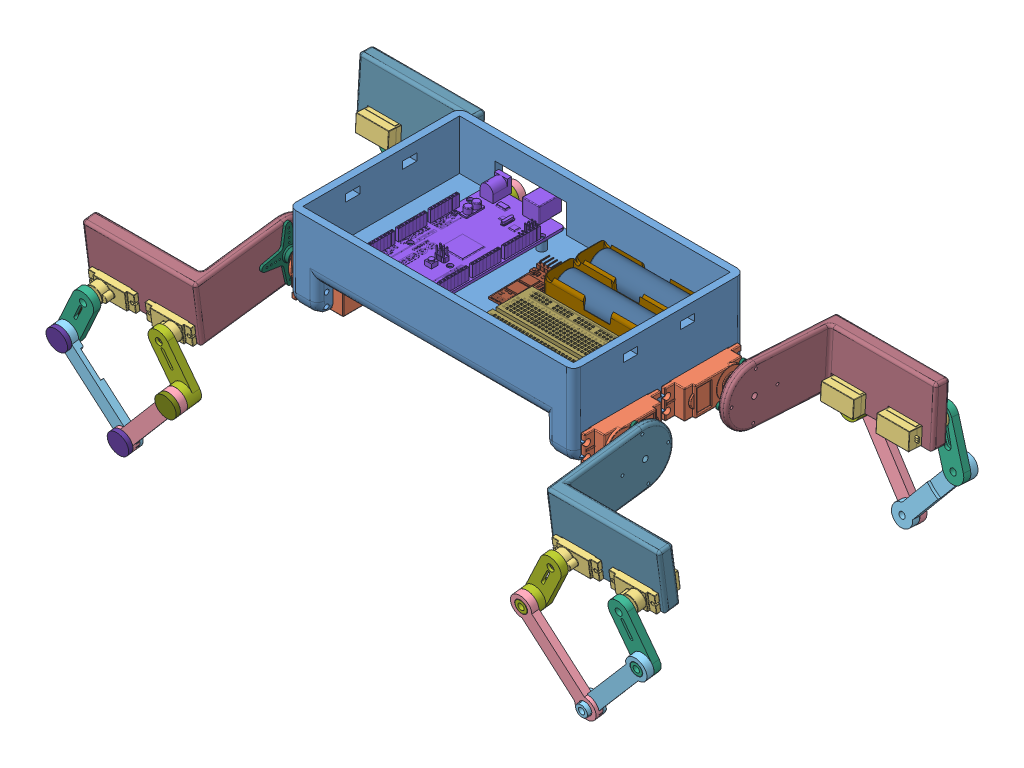
SolidWorks assembly ASSY2, configuration Default. Lengths in mm.
Overall size (425 157.55 250.82).
49 component instances, 18 part files, 74 mates.
Components (placement in the parent):
- part1-1: part1 [Default] at (0 551.341 0) size (200.21 60 120)
- Servo MG996R-2: Servo MG996R [Predeterminado] at (-73.4 551.341 48.3) x (0 0 -1) z (0 1 0) size (53.6 47.6 20)
- Servo-MG90S-1: Servo-MG90S [Default] at (-142.75 521.5824 79.9275) x (1 0 0) z (0 -0.991575 -0.129534) size (32.2 32.5 12.4)
- Servo-MG90S-2: Servo-MG90S [Default] at (-182.75 521.5824 79.9275) x (-1 0 0) z (0 0.991575 0.129534) size (32.2 32.5 12.4)
- legpart1-1: legpart1 [Default] at (-123.3346 490.3083 115.1734) x (-0.653604 -0.75046 -0.098036) z (0 -0.129534 0.991575) size (75 15 5)
- legpart2-1: legpart2 [Default] at (-201.9182 490.4764 112.8758) x (0.656123 -0.748296 -0.097754) z (0 -0.129534 0.991575) size (75 15 10)
- legpart3-1: legpart3 [Default] at (-188 517.4761 111.3604) x (-0.46394 -0.878403 -0.11475) z (0 -0.129534 0.991575) size (45 15 10)
- legpart4-1: legpart4 [Default] at (-137.5 517.8259 108.6831) x (0.472181 -0.874075 -0.114185) z (0 -0.129534 0.991575) size (45 15 15.1)
- Arduino Mega.step-1: Arduino Mega.step [Default] at (-11.5076 562.341 34.714) x (0.34202 0 -0.939693) z (0.939693 0 0.34202) size (114.59 14.37 81.93)
  - ARDUINO MEGA_1.step-1: ARDUINO MEGA_1.step [Default] at origin size (114.59 14.37 81.93)
- 18650BatteryCase v6.step-1: 18650BatteryCase v6.step [Default] at (12.6809 556.341 -27.3839) x (1 0 0) z (0 1 0) size (76.1 23.18 18.4)
- 18650 battery-1: 18650 battery [Default] at (82.6809 566.341 -39.3839) x (0 0 1) z (0 -1 0) size (18.4 65 18.4)
- 18650 battery-3: 18650 battery [Default] at (82.6809 566.341 -15.3839) x (0 0 -1) z (0 1 0) size (18.4 65 18.4)
- 18650BatteryCase v6.step-3: 18650BatteryCase v6.step [Default] at (12.6809 556.341 -5.8839) x (1 0 0) z (0 1 0) size (76.1 23.18 18.4)
- HC-05-1: HC-05 [Default] at (-0.9997 556.341 -7.5776) x (-0.021576 0 -0.999767) z (0.999767 0 -0.021576) size (42.58 6.55 16)
- matrix-1: matrix [Default] at (54 556.341 28.5) size (82 14.01 53)
- part2L-7: part2L [Default] at (-125.75 541.341 38.3) x (0 -0.129534 0.991575) z (-1 0 0) size (82.34 40 80)
- part2R-7: part2R [Default] at (-125.75 541.341 -38.3) x (0 -0.058757 -0.998272) z (-1 0 0) size (82.34 40 80)
- Servo MG996R-8: Servo MG996R [Predeterminado] at (-73.4 531.341 -48.3) x (0 0 1) z (0 -1 0) size (53.6 47.6 20)
- Servo MG996R-9: Servo MG996R [Predeterminado] at (73.4 551.341 -48.3) x (0 0 1) z (0 1 0) size (53.6 47.6 20)
- Servo MG996R-10: Servo MG996R [Predeterminado] at (73.4 531.341 48.3) x (0 0 -1) z (0 -1 0) size (53.6 47.6 20)
- Servo Control Horns-1: Servo Control Horns [4 Arm] at (-121 531.0968 37.9577) x (0 -0.999442 -0.033391) z (-1 0 0) size (39 39 5.5)
- Servo Control Horns-2: Servo Control Horns [4 Arm] at (-121 540.9638 -28.057) x (0 -0.036806 0.999322) z (-1 0 0) size (39 39 5.5)
- Servo-MG90S-13: Servo-MG90S [Default] at (-182.75 524.5899 -81.2261) x (-1 0 0) z (0 -0.998272 0.058757) size (32.2 32.5 12.4)
- Servo-MG90S-14: Servo-MG90S [Default] at (-143.75 524.5899 -81.2261) x (1 0 0) z (0 0.998272 -0.058757) size (32.2 32.5 12.4)
- legpart4-8: legpart4 [Default] at (-138.5 522.8859 -110.176) x (0.476344 -0.87774 0.051662) z (0 -0.058757 -0.998272) size (45 15 15.1)
- legpart1-8: legpart1 [Default] at (-124.2097 495.6724 -123.6002) x (-0.593927 -0.803129 0.047271) z (0 0.058757 0.998272) size (75 15 5)
- legpart2-8: legpart2 [Default] at (-197.9499 494.3391 -113.5044) x (0.635076 -0.771115 0.045387) z (0 -0.058757 -0.998272) size (75 15 10)
- legpart3-8: legpart3 [Default] at (-188 522.8859 -110.176) x (-0.331664 -0.941768 0.055431) z (0 -0.058757 -0.998272) size (45 15 10)
- Servo Control Horns-3: Servo Control Horns [4 Arm] at (121 551.5745 -37.7196) x (0 0.998396 0.056621) z (1 0 0) size (39 39 5.5)
- Servo Control Horns-5: Servo Control Horns [4 Arm] at (121 541.7183 28.057) x (0 0.036806 -0.999322) z (1 0 0) size (39 39 5.5)
- part2R-12: part2R [Default] at (125.75 541.341 38.3) x (0 -0.129534 0.991575) z (1 0 0) size (82.34 40 80)
- part2L-13: part2L [Default] at (125.75 541.341 -38.3) x (0 -0.058757 -0.998272) z (1 0 0) size (82.34 40 80)
- legpart4-14: legpart4 [Default] at (138.5 522.8859 -110.176) x (-0.476344 -0.87774 0.051662) z (0 -0.058757 -0.998272) size (45 15 15.1)
- legpart3-14: legpart3 [Default] at (188 522.8859 -110.176) x (0.331664 -0.941768 0.055431) z (0 -0.058757 -0.998272) size (45 15 10)
- Servo-MG90S-25: Servo-MG90S [Default] at (182.75 524.5899 -81.2261) x (1 0 0) z (0 0.998272 -0.058757) size (32.2 32.5 12.4)
- Servo-MG90S-26: Servo-MG90S [Default] at (143.75 524.5899 -81.2261) x (-1 0 0) z (0 -0.998272 0.058757) size (32.2 32.5 12.4)
- legpart1-14: legpart1 [Default] at (124.2097 495.9662 -118.6089) x (0.593927 -0.803129 0.047271) z (0 -0.058757 -0.998272) size (75 15 5)
- legpart2-14: legpart2 [Default] at (197.9499 494.3391 -113.5044) x (-0.635076 -0.771115 0.045387) z (0 -0.058757 -0.998272) size (75 15 10)
- Servo-MG90S-27: Servo-MG90S [Default] at (142.75 521.5824 79.9275) x (-1 0 0) z (0 0.991575 0.129534) size (32.2 32.5 12.4)
- Servo-MG90S-28: Servo-MG90S [Default] at (182.75 521.5824 79.9275) x (1 0 0) z (0 -0.991575 -0.129534) size (32.2 32.5 12.4)
- legpart3-15: legpart3 [Default] at (188 517.4761 111.3604) x (0.46394 -0.878403 -0.11475) z (0 -0.129534 0.991575) size (45 15 10)
- legpart2-15: legpart2 [Default] at (201.9182 490.4764 112.8758) x (-0.656123 -0.748296 -0.097754) z (0 -0.129534 0.991575) size (75 15 10)
- legpart1-15: legpart1 [Default] at (123.3346 489.6606 120.1312) x (0.653604 -0.75046 -0.098036) z (0 0.129534 -0.991575) size (75 15 5)
- legpart4-15: legpart4 [Default] at (137.5 517.8259 108.6831) x (-0.472181 -0.874075 -0.114185) z (0 -0.129534 0.991575) size (45 15 15.1)
- legpart5-1: legpart5 [Default] at (-123.3346 489.272 123.106) x (-0.914565 -0.401032 -0.052389) z (0.40444 -0.906859 -0.118467) size (15 18 15)
- legpart6-1: legpart6 [Default] at (-162.5508 444.2444 117.2238) x (0.999961 0.008715 0.001138) z (-0.008789 0.991537 0.129529) size (15 13 15)
- legpart6-2: legpart6 [Default] at (-201.9182 489.4401 120.8084) x (0.324849 0.937798 0.122509) z (-0.945766 0.322112 0.042079) size (15 13 15)
- servo horn 1 v2.step-1: servo horn 1 v2.step [Default] at (-188 517.3725 112.1537) x (0.877073 -0.476309 -0.062223) z (-0.480356 -0.869684 -0.113611) size (7.2 3.7 21.2)
Mates (geometry in assembly coordinates):
- 일치5: coincident: plane of part1-1 through (0 551.341 0) normal (0 -1 0); plane of Servo MG996R-2 through (-110 551.341 48.3) normal (0 1 0)
- 일치22: coincident: plane of Servo-MG90S-1 through (-137.5 517.8259 108.6831) normal (0 -0.129534 0.991575); plane of legpart4-1 through (-137.5 517.8259 108.6831) normal (0 0.129534 -0.991575)
- 동심5: concentric: cylinder of Servo-MG90S-1 through (-137.5 517.6963 109.6747) axis (0 -0.129534 0.991575) radius 1.25; cylinder of legpart4-1 through (-137.5 517.1782 113.641) axis (0 0.129534 -0.991575) radius 2.5
- 동심6: concentric: cylinder of legpart1-1 through (-123.3346 489.6606 120.1312) axis (0 0.129534 -0.991575) radius 4.5; cylinder of legpart4-1 through (-123.3346 489.6476 120.2304) axis (0 0.129534 -0.991575) radius 4.25
- 일치23: coincident: plane of legpart1-1 through (-123.3346 490.3083 115.1734) normal (0 0.129534 -0.991575); plane of legpart4-1 through (-123.3346 490.3083 115.1734) normal (0 -0.129534 0.991575)
- 동심7: concentric: cylinder of Servo-MG90S-2 through (-188 517.6963 109.6747) axis (0 -0.129534 0.991575) radius 1.25; cylinder of legpart3-1 through (-188 516.8285 116.3183) axis (0 0.129534 -0.991575) radius 2.5
- 동심8: concentric: cylinder of legpart2-1 through (-201.9182 489.8287 117.8336) axis (0 0.129534 -0.991575) radius 4.5; cylinder of legpart3-1 through (-201.9182 489.8287 117.8336) axis (0 0.129534 -0.991575) radius 4.25
- 일치25: coincident: plane of legpart2-1 through (-201.9182 490.4764 112.8758) normal (0 0.129534 -0.991575); plane of legpart3-1 through (-188 516.8285 116.3183) normal (0 -0.129534 0.991575)
- 동심9: concentric: cylinder of legpart1-1 through (-162.5508 444.633 114.2491) axis (0 0.129534 -0.991575) radius 4.5; cylinder of legpart2-1 through (-162.5508 444.2832 116.9263) axis (0 0.129534 -0.991575) radius 4.25
- 거리7: distance = 20 mm: plane of Arduino Mega.step-1/ARDUINO MEGA_1.step-1 through (-40 564.141 -52) normal (-1 0 0); plane of part1-1 through (-20 576.341 -45) normal (-1 0 0)
- 일치31: coincident: plane of part1-1 through (0 556.341 0) normal (0 1 0); plane of 18650BatteryCase v6.step-1 through (50.6809 556.341 -38.1339) normal (0 -1 0)
- 거리8: distance = 10 mm: plane of 18650BatteryCase v6.step-1 through (12.6809 556.341 -27.3839) normal (0 1 0); plane of 18650 battery-1 through (82.6809 566.341 -39.3839) normal (0 -1 0)
- 거리9: distance = 12 mm: plane of 18650 battery-1 through (82.6809 566.341 -39.3839) normal (0 0 1); plane of 18650BatteryCase v6.step-1 through (12.6809 556.341 -27.3839) normal (0 0 -1)
- 거리10: distance = 70 mm: plane of 18650 battery-1 through (82.6809 566.341 -39.3839) normal (-1 0 0); plane of 18650BatteryCase v6.step-1 through (12.6809 556.341 -27.3839) normal (1 0 0)
- 일치33: coincident: plane of part1-1 through (0 556.341 0) normal (0 1 0); plane of matrix-1 through (54 556.341 28.5) normal (0 -1 0)
- 일치34: coincident: plane of part1-1 through (95 591.341 -55) normal (-1 0 0); plane of matrix-1 through (95 570.3451 2) normal (1 0 0)
- 일치35: coincident: plane of part1-1 through (-95 591.341 55) normal (0 0 -1); plane of matrix-1 through (95 570.3451 55) normal (0 0 1)
- 일치36: coincident: plane of part1-1 through (0 556.341 0) normal (0 1 0); plane of HC-05-1 through (-0.9997 556.341 -7.5776) normal (0 -1 0)
- 일치38: coincident: plane of part1-1 through (0 551.341 0) normal (1 0 0); plane of assembly through (0 0 0) normal (1 0 0)
- 일치39: coincident: plane of part1-1 through (-100 556.341 -60) normal (0 0 -1); plane of Arduino Mega.step-1/ARDUINO MEGA_1.step-1 through (-34 564.641 -60) normal (0 0 -1)
- 일치40: coincident: plane of part1-1 through (-62.5 562.341 12.1502) normal (0 1 0); plane of Arduino Mega.step-1/ARDUINO MEGA_1.step-1 through (-44 562.341 -52) normal (0 -1 0)
- 일치42: coincident: plane of Servo-MG90S-2 through (-182.75 519.186 98.2716) normal (0 0.129534 -0.991575); plane of part2L-7 through (-125.75 533.2663 100.111) normal (0 -0.129534 0.991575)
- 일치44: coincident: plane of Servo-MG90S-2 through (-182.75 527.7301 80.7306) normal (0 0.991575 0.129534); plane of part2L-7 through (-194.75 526.6291 89.159) normal (0 -0.991575 -0.129534)
- 일치45: coincident: plane of Servo-MG90S-1 through (-142.75 527.7301 80.7306) normal (0 0.991575 0.129534); plane of part2L-7 through (-130.75 526.6291 89.159) normal (0 -0.991575 -0.129534)
- 일치46: coincident: plane of Servo-MG90S-1 through (-142.75 519.186 98.2716) normal (0 0.129534 -0.991575); plane of part2L-7 through (-125.75 533.2663 100.111) normal (0 -0.129534 0.991575)
- 거리11: distance = 0.5 mm: plane of Servo-MG90S-1 through (-154.25 513.2365 97.4944) normal (-1 0 0); plane of part2L-7 through (-154.75 514.7302 87.6046) normal (1 0 0)
- 거리12: distance = 0.5 mm: plane of part2L-7 through (-194.75 514.7302 87.6046) normal (1 0 0); plane of Servo-MG90S-2 through (-194.25 525.1354 99.0488) normal (-1 0 0)
- 동심14: concentric: cylinder of Servo MG996R-2 through (-114.1 541.341 38.3) axis (-1 0 0) radius 1.3; cylinder of Servo Control Horns-1 through (-122.75 541.341 38.3) axis (1 0 0) radius 1.25
- 일치47: coincident: plane of Servo MG996R-2 through (-121 541.341 38.3) normal (-1 0 0); plane of Servo Control Horns-1 through (-121 531.0968 37.9577) normal (1 0 0)
- 일치48: coincident: plane of part2L-7 through (-122.75 541.341 38.3) normal (1 0 0); plane of Servo Control Horns-1 through (-122.75 531.0968 37.9577) normal (-1 0 0)
- 동심16: concentric: cylinder of part2L-7 through (-122.75 541.341 38.3) axis (-1 0 0) radius 2; cylinder of Servo Control Horns-1 through (-122.75 541.341 38.3) axis (1 0 0) radius 1.25
- 동심17: concentric: cylinder of Servo MG996R-8 through (-114.1 541.341 -38.3) axis (-1 0 0) radius 1.3; cylinder of Servo Control Horns-2 through (-122.75 541.341 -38.3) axis (1 0 0) radius 1.25
- 일치49: coincident: plane of Servo MG996R-8 through (-121 541.341 -38.3) normal (-1 0 0); plane of Servo Control Horns-2 through (-121 540.9638 -28.057) normal (1 0 0)
- 동심18: concentric: cylinder of part2R-7 through (-122.75 541.341 -38.3) axis (-1 0 0) radius 2; cylinder of Servo Control Horns-2 through (-122.75 541.341 -38.3) axis (1 0 0) radius 1.25
- 일치50: coincident: plane of part2R-7 through (-122.75 541.341 -38.3) normal (1 0 0); plane of Servo Control Horns-2 through (-122.75 540.9638 -28.057) normal (-1 0 0)
- 일치51: coincident: plane of Servo-MG90S-14 through (-138.5 522.8859 -110.176) normal (0 -0.058757 -0.998272); plane of legpart4-8 through (-138.5 522.8859 -110.176) normal (0 0.058757 0.998272)
- 동심19: concentric: cylinder of Servo-MG90S-14 through (-138.5 522.8272 -111.1743) axis (0 -0.058757 -0.998272) radius 1.25; cylinder of legpart4-8 through (-138.5 522.5922 -115.1674) axis (0 0.058757 0.998272) radius 2.5
- 동심20: concentric: cylinder of legpart4-8 through (-124.2097 495.6665 -123.7) axis (0 0.058757 0.998272) radius 4.25; cylinder of legpart1-8 through (-124.2097 495.9662 -118.6089) axis (0 -0.058757 -0.998272) radius 4.5
- 일치52: coincident: plane of legpart4-8 through (-124.2097 495.9662 -118.6089) normal (0 -0.058757 -0.998272); plane of legpart1-8 through (-124.2097 495.9662 -118.6089) normal (0 0.058757 0.998272)
- 일치53: coincident: plane of Servo-MG90S-13 through (-188 522.8859 -110.176) normal (0 -0.058757 -0.998272); plane of legpart3-8 through (-188 522.8859 -110.176) normal (0 0.058757 0.998272)
- 동심21: concentric: cylinder of Servo-MG90S-13 through (-188 522.8272 -111.1743) axis (0 -0.058757 -0.998272) radius 1.25; cylinder of legpart3-8 through (-188 522.5922 -115.1674) axis (0 0.058757 0.998272) radius 2.5
- 동심22: concentric: cylinder of legpart2-8 through (-197.9499 494.0453 -118.4958) axis (0 0.058757 0.998272) radius 4.5; cylinder of legpart3-8 through (-197.9499 494.0453 -118.4958) axis (0 0.058757 0.998272) radius 4.25
- 일치54: coincident: plane of legpart2-8 through (-197.9499 494.3391 -113.5044) normal (0 0.058757 0.998272); plane of legpart3-8 through (-188 522.5922 -115.1674) normal (0 -0.058757 -0.998272)
- 동심23: concentric: cylinder of legpart1-8 through (-159.8453 447.7784 -115.7726) axis (0 -0.058757 -0.998272) radius 4.5; cylinder of legpart2-8 through (-159.8453 447.4847 -120.764) axis (0 0.058757 0.998272) radius 4.25
- 일치55: coincident: plane of part2R-7 through (-130.75 530.2797 -90.0757) normal (0 -0.998272 0.058757); plane of Servo-MG90S-14 through (-143.75 530.7792 -81.5904) normal (0 0.998272 -0.058757)
- 거리13: distance = 0.5 mm: plane of Servo-MG90S-14 through (-155.25 529.4925 -100.0467) normal (-1 0 0); plane of part2R-7 through (-154.75 530.2797 -90.0757) normal (1 0 0)
- 일치56: coincident: plane of part2R-7 through (-130.75 530.2797 -90.0757) normal (0 -0.998272 0.058757); plane of Servo-MG90S-14 through (-143.75 530.7792 -81.5904) normal (0 0.998272 -0.058757)
- 일치57: coincident: plane of part2R-7 through (-125.75 537.6783 -100.5285) normal (0 -0.058757 -0.998272); plane of Servo-MG90S-14 through (-143.75 523.5029 -99.6941) normal (0 0.058757 0.998272)
- 거리14: distance = 0.5 mm: plane of Servo-MG90S-13 through (-194.25 517.5132 -99.3416) normal (-1 0 0); plane of part2R-7 through (-194.75 530.2797 -90.0757) normal (1 0 0)
- 일치58: coincident: plane of part2R-7 through (-194.75 530.2797 -90.0757) normal (0 -0.998272 0.058757); plane of Servo-MG90S-13 through (-182.75 530.7792 -81.5904) normal (0 0.998272 -0.058757)
- 일치59: coincident: plane of part2R-7 through (-125.75 537.6783 -100.5285) normal (0 -0.058757 -0.998272); plane of Servo-MG90S-13 through (-182.75 523.5029 -99.6941) normal (0 0.058757 0.998272)
- 동심33: concentric: cylinder of Servo Control Horns-3 through (122.75 541.341 -38.3) axis (-1 0 0) radius 1.25; cylinder of part2L-13 through (122.75 541.341 -38.3) axis (1 0 0) radius 2
- 동심35: concentric: cylinder of Servo Control Horns-5 through (122.75 541.341 38.3) axis (-1 0 0) radius 1.25; cylinder of part2R-12 through (122.75 541.341 38.3) axis (1 0 0) radius 2
- 동심37: concentric: cylinder of Servo MG996R-10 through (114.1 541.341 38.3) axis (1 0 0) radius 1.3; cylinder of Servo Control Horns-5 through (122.75 541.341 38.3) axis (-1 0 0) radius 1.25
- 일치71: coincident: plane of Servo MG996R-10 through (121 541.341 38.3) normal (1 0 0); plane of Servo Control Horns-5 through (121 541.7183 28.057) normal (-1 0 0)
- 동심38: concentric: cylinder of Servo MG996R-9 through (114.1 541.341 -38.3) axis (1 0 0) radius 1.3; cylinder of Servo Control Horns-3 through (122.75 541.341 -38.3) axis (-1 0 0) radius 1.25
- 일치72: coincident: plane of Servo MG996R-9 through (121 541.341 -38.3) normal (1 0 0); plane of Servo Control Horns-3 through (121 551.5745 -37.7196) normal (-1 0 0)
- 일치73: coincident: plane of Servo Control Horns-3 through (122.75 551.5745 -37.7196) normal (1 0 0); plane of part2L-13 through (122.75 541.341 -38.3) normal (-1 0 0)
- 일치74: coincident: plane of part2L-13 through (130.75 530.2797 -90.0757) normal (0 -0.998272 0.058757); plane of Servo-MG90S-26 through (143.75 530.7792 -81.5904) normal (0 0.998272 -0.058757)
- 일치75: coincident: plane of part2R-12 through (130.75 526.6291 89.159) normal (0 -0.991575 -0.129534); plane of Servo-MG90S-27 through (142.75 527.7301 80.7306) normal (0 0.991575 0.129534)
- 일치76: coincident: plane of Servo Control Horns-5 through (122.75 541.7183 28.057) normal (1 0 0); plane of part2R-12 through (122.75 541.341 38.3) normal (-1 0 0)
- 일치77: coincident: plane of part1-1 through (0 551.341 0) normal (0 -1 0); plane of Servo MG996R-8 through (-110 551.341 -48.3) normal (0 1 0)
- 거리16: distance = 0.5 mm: plane of Servo MG996R-2 through (-110 551.341 8) normal (0 0 -1); plane of part1-1 through (0 531.341 7.5) normal (0 0 1)
- 거리17: distance = 0.5 mm: plane of Servo MG996R-8 through (-110 531.341 -8) normal (0 0 1); plane of part1-1 through (0 531.341 -7.5) normal (0 0 -1)
- 동심40: concentric: cylinder of legpart4-1 through (-123.3346 494.3238 84.4345) axis (0 -0.129534 0.991575) radius 2.25; cylinder of legpart5-1 through (-123.3346 491.6036 105.2576) axis (0 -0.129534 0.991575) radius 2
- 일치84: coincident: plane of legpart1-1 through (-123.3346 489.6606 120.1312) normal (0 -0.129534 0.991575); plane of legpart5-1 through (-123.3346 489.6606 120.1312) normal (0 0.129534 -0.991575)
- 동심42: concentric: cylinder of legpart2-1 through (-162.5508 446.6149 99.078) axis (0 -0.129534 0.991575) radius 2.25; cylinder of legpart6-1 through (-162.5508 445.9283 104.3333) axis (0 -0.129534 0.991575) radius 2
- 일치86: coincident: plane of legpart1-1 through (-123.3346 489.6606 120.1312) normal (0 -0.129534 0.991575); plane of legpart6-1 through (-162.5508 444.633 114.2491) normal (0 0.129534 -0.991575)
- 동심43: concentric: cylinder of legpart3-1 through (-201.9182 495.0101 78.1706) axis (0 -0.129534 0.991575) radius 2.25; cylinder of legpart6-2 through (-201.9182 491.124 107.9179) axis (0 -0.129534 0.991575) radius 2
- 일치87: coincident: plane of legpart2-1 through (-201.9182 489.8287 117.8336) normal (0 -0.129534 0.991575); plane of legpart6-2 through (-201.9182 489.8287 117.8336) normal (0 0.129534 -0.991575)
- 일치88: coincident: plane of part1-1 through (-100 556.341 -60) normal (-1 0 0); plane of Servo MG996R-2 through (-100 551.341 54.95) normal (1 0 0)
- 일치90: coincident: plane of Servo-MG90S-2 through (-188 517.3725 112.1537) normal (0 -0.129534 0.991575); plane of servo horn 1 v2.step-1 through (-188 517.3725 112.1537) normal (0 0.129534 -0.991575)
- 동심44: concentric: cylinder of Servo-MG90S-2 through (-188 517.6963 109.6747) axis (0 -0.129534 0.991575) radius 1.25; cylinder of servo horn 1 v2.step-1 through (-188 517.3725 112.1537) axis (0 -0.129534 0.991575) radius 1.1
- 일치91: coincident: plane of legpart3-1 through (-195.423 503.1626 111.5075) normal (0 0.129534 -0.991575); plane of servo horn 1 v2.step-1 through (-191.3625 511.1293 112.5483) normal (0 -0.129534 0.991575)
